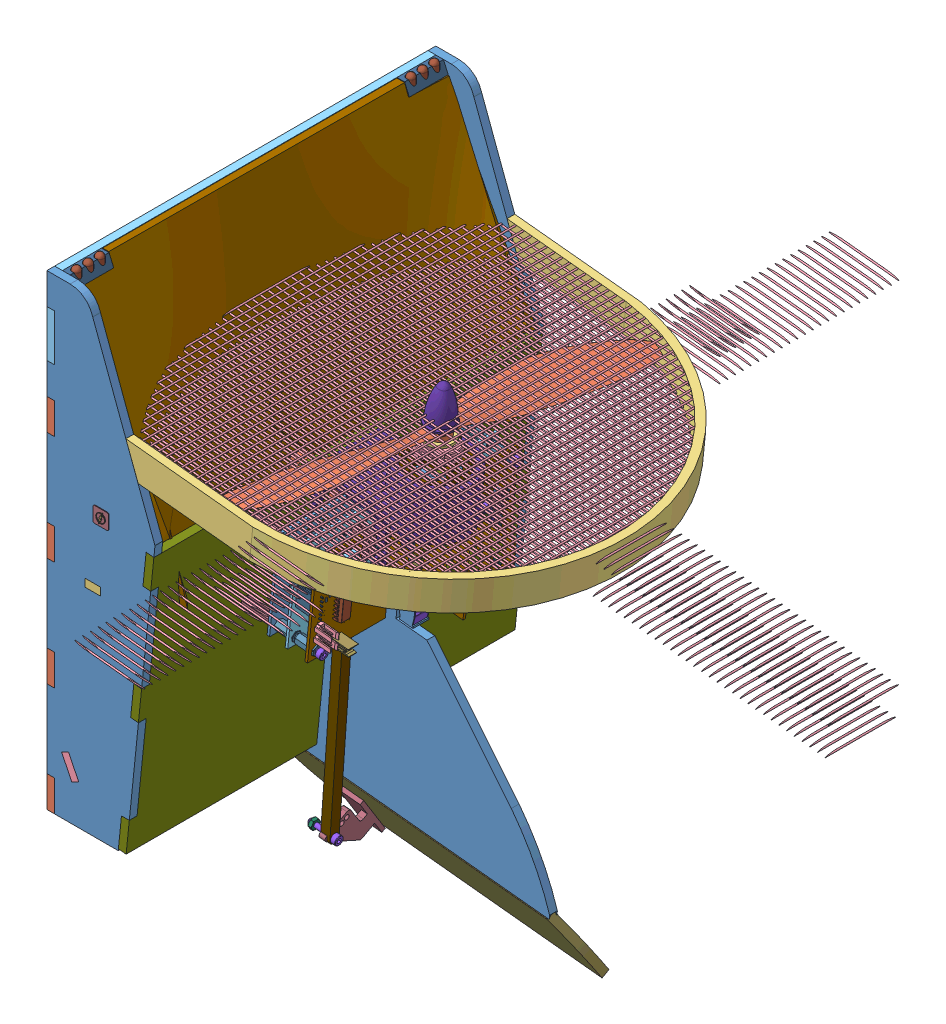
SolidWorks assembly AssTotaleSimu2, configuration Défaut. Lengths in mm. (continued)
Components (placement in the parent): (continued)
- AssStructSimu-1: AssStructSimu [Défaut] at (-125.7658 -1.8483 624.6548) x (1 0 0) z (0 0 -1) size (253.25 324.59 251.6) (continued)
  - AssCarte-1: AssCarte [Défaut] at (38.0121 147.1029 290.772) x (-0.101852 0.9948 0) z (0.9948 0.101852 0) size (66.52 130.57 98.72) (continued)
    - carte_onduleur_v3-1: carte_onduleur_v3 [Défaut] at (-131.8199 12.0892 20.7912) size (66.52 130.57 82.34) (continued)
      - U_DSPIC-1: U_DSPIC [Défaut] at (1.863 -2.61 0.803) size (7.92 35.56 7.75)
        - Open CASCADE STEP translator 6.8 1.17.1-1: Open CASCADE STEP translator 6.8 1.17.1 [Défaut] at origin size (7.92 35.56 7.75)
          - Body_1_4-1: Body_1_4 [Défaut] at (0 -0.2 4) x (1 0 0) z (0 -1 0) size (7.92 7.75 35.56)
      - C_DEC_DSPIC-1: C_DEC_DSPIC [Défaut] at (7.7 -8.8 -0.803) x (0 1 0) z (0 0 -1) size (2.34 1.04 0.5)
        - Open CASCADE STEP translator 6.8 1.6.1-1: Open CASCADE STEP translator 6.8 1.6.1 [Défaut] at origin size (2.34 1.04 0.5)
          - Body_1-1: Body_1 [Défaut] at origin size (2.29 1.04 0.43)
          - Pin_1-1: Pin_1 [Défaut] at (0.3048 0 0) x (-1 0 0) z (0 0 1) size (0.51 1.02 0.5)
          - Pin_2-1: Pin_2 [Défaut] at origin size (0.51 1.02 0.5)
      - IN-1: IN [Défaut] at (24.3 -5.3 0.803) x (0 1 0) z (0 0 1) size (10.21 15.56 26.9)
        - Open CASCADE STEP translator 6.8 1.19.1-1: Open CASCADE STEP translator 6.8 1.19.1 [Défaut] at origin size (10.21 15.56 26.9)
          - Body_1_3-1: Body_1_3 [Défaut] at (-13.5 1.8 3) x (0 1 0) z (1 0 0) size (15.56 26.9 10.21)
            - Imported-1: Imported [Défaut] at (2.0451 -4.5908 20.9802) size (8.6 15.9 10.16)
            - Imported-2: Imported [Défaut] at (-1.6683 9.1092 15.9802) x (0 0 1) z (-1 0 0) size (10.1 18.2 15.1)
              - Imported_2-1: Imported_2 [Défaut] at origin size (10.1 18.2 15.1)
              - Imported_3-1: Imported_3 [Défaut] at origin size (3.43 12.4 4.99)
              - Imported_4-1: Imported_4 [Défaut] at origin size (3.43 12.4 4.99)
              - Imported_5-1: Imported_5 [Défaut] at origin size (3.9 4.9 7)
              - Imported_6-1: Imported_6 [Défaut] at origin size (3.9 4.9 7)
              - Imported_7-1: Imported_7 [Défaut] at origin size (3.8 3.8 6.92)
              - Imported_8-1: Imported_8 [Défaut] at origin size (3.8 3.8 6.92)
              - Imported_9-1: Imported_9 [Défaut] at origin size (9 2.4 14.2)
      - CARTE_CMD-1: CARTE_CMD [Défaut] at (25 57.2 0.803) size (60.1 130 26.71)
        - Open CASCADE STEP translator 6.8 1.20.1-1: Open CASCADE STEP translator 6.8 1.20.1 [Défaut] at origin size (60.1 130 26.71)
          - Body_1_4-1: Body_1_4 [Défaut] at (-55 5 12) size (60.1 130 26.71)
            - 1_2-1: 1_2 [Défaut] at origin size (60.1 130 1.61)
            - 4-1: 4 [Défaut] at (23.6 -124.9 0.803) x (0 1 0) z (0 0 1) size (5 15.24 14.3)
              - =_[0_1_1_4]_2-1: =_[0_1_1_4]_2 [Défaut] at origin size (5 15.24 14.3)
                - 5-1: 5 [Défaut] at (0 -6.5 -13) x (0 1 0) z (0 0 -1) size (15.24 5 14.3)
            - 7-1: 7 [Défaut] at (23.6 -5 0.803) x (0 1 0) z (0 0 1) size (5 15.24 14.3)
              - =_[0_1_1_7]-1: =_[0_1_1_7] [Défaut] at origin size (5 15.24 14.3)
                - 5-1: 5 [Défaut] at (0 -6.5 -13) x (0 1 0) z (0 0 -1) size (15.24 5 14.3)
            - 10_2-1: 10_2 [Défaut] at (18.4 -115.6 0.803) size (25.4 7.92 7.75)
              - =_[0_1_1_9]-1: =_[0_1_1_9] [Défaut] at origin size (25.4 7.92 7.75)
                - 8-1: 8 [Défaut] at (11.2 4 0) x (0 1 0) z (1 0 0) size (7.92 7.75 25.4)
            - 13_2-1: 13_2 [Défaut] at (55.4 -114.7 0.803) x (-1 0 0) z (0 0 1) size (5 7.62 14.3)
              - =_[0_1_1_12]-1: =_[0_1_1_12] [Défaut] at origin size (5 7.62 14.3)
                - 11-1: 11 [Défaut] at (0 -2.5 11) x (0 -1 0) z (0 0 1) size (7.62 5 14.3)
            - 25-1: 25 [Défaut] at (56.9 -12.8 0.803) x (-1 0 0) z (0 0 1) size (16.02 47.26 11.05)
              - =_[0_1_1_15]_2-1: =_[0_1_1_15]_2 [Défaut] at origin size (16.02 47.26 11.05)
                - 23-1: 23 [Défaut] at (-36.5 21 4) x (0 -1 0) z (1 0 0) size (47.26 11.05 16.02)
                  - 14-1: 14 [Défaut] at (-7.4961 -1.5352 42.5833) size (42.58 6.55 16.01)
                  - 22-1: 22 [Défaut] at (19.3039 2.3748 37.905) x (-1 0 0) z (0 0 -1) size (10.36 6.14 15.24)
                    - 21-1: 21 [Défaut] at origin size (10.36 6.14 7.62)
                      - 19_2-1: 19_2 [Défaut] at origin size (10.36 6.14 2.54)
                        - 15-1: 15 [Défaut] at origin size (8.4 2.54 2.54)
                        - 16-1: 16 [Défaut] at (-0.0461 1.2682 1.27) x (0 0 -1) z (0.999998 -0.002105 0) size (1.95 5.07 7.58)
                      - 19_2-2: 19_2 [Défaut] at (0 0 -2.54) size (10.36 6.14 2.54)
                        - 15-1: 15 [Défaut] at origin size (8.4 2.54 2.54)
                        - 16-1: 16 [Défaut] at (-0.0461 1.2682 1.27) x (0 0 -1) z (0.999998 -0.002105 0) size (1.95 5.07 7.58)
                      - 19_2-3: 19_2 [Défaut] at (0 0 -5.08) size (10.36 6.14 2.54)
                        - 15-1: 15 [Défaut] at origin size (8.4 2.54 2.54)
                        - 16-1: 16 [Défaut] at (-0.0461 1.2682 1.27) x (0 0 -1) z (0.999998 -0.002105 0) size (1.95 5.07 7.58)
                    - 21-2: 21 [Défaut] at (0 0 -7.62) size (10.36 6.14 7.62)
                      - 19_2-1: 19_2 [Défaut] at origin size (10.36 6.14 2.54)
                        - 15-1: 15 [Défaut] at origin size (8.4 2.54 2.54)
                        - 16-1: 16 [Défaut] at (-0.0461 1.2682 1.27) x (0 0 -1) z (0.999998 -0.002105 0) size (1.95 5.07 7.58)
                      - 19_2-2: 19_2 [Défaut] at (0 0 -2.54) size (10.36 6.14 2.54)
                        - 15-1: 15 [Défaut] at origin size (8.4 2.54 2.54)
                        - 16-1: 16 [Défaut] at (-0.0461 1.2682 1.27) x (0 0 -1) z (0.999998 -0.002105 0) size (1.95 5.07 7.58)
                      - 19_2-3: 19_2 [Défaut] at (0 0 -5.08) size (10.36 6.14 2.54)
                        - 15-1: 15 [Défaut] at origin size (8.4 2.54 2.54)
                        - 16-1: 16 [Défaut] at (-0.0461 1.2682 1.27) x (0 0 -1) z (0.999998 -0.002105 0) size (1.95 5.07 7.58)
            - 31-1: 31 [Défaut] at (12.9 -104.5 0.803) size (6.76 3.64 4.37)
              - =_[0_1_1_24]-1: =_[0_1_1_24] [Défaut] at origin size (6.76 3.64 4.37)
                - 29-1: 29 [Défaut] at (-0.3 -2 0) size (6.76 3.64 4.37)
                  - =_[0_1_1_3]_3-1: =_[0_1_1_3]_3 [Défaut] at origin size (6 3.64 4.37)
                  - =_[0_1_1_4]_3-1: =_[0_1_1_4]_3 [Défaut] at origin size (0.38 1 0.67)
                  - =_[0_1_1_5]_3-1: =_[0_1_1_5]_3 [Défaut] at origin size (0.38 1 0.67)
            - 36-1: 36 [Défaut] at (28.6 -12.2 0.803) x (0 -1 0) z (0 0 1) size (2.34 1.04 0.5)
              - =_[0_1_1_30]-1: =_[0_1_1_30] [Défaut] at origin size (2.34 1.04 0.5)
                - 32_2-1: 32_2 [Défaut] at origin size (2.29 1.04 0.43)
                - 33_2-1: 33_2 [Défaut] at (0.3048 0 0) x (-1 0 0) z (0 0 1) size (0.51 1.02 0.5)
                - 34-1: 34 [Défaut] at origin size (0.51 1.02 0.5)
            - 38-1: 38 [Défaut] at (23.7 -12.2 0.803) x (0 -1 0) z (0 0 1) size (2.34 1.04 0.5)
              - =_[0_1_1_30]-1: =_[0_1_1_30] [Défaut] at origin size (2.34 1.04 0.5)
                - 32_2-1: 32_2 [Défaut] at origin size (2.29 1.04 0.43)
                - 33_2-1: 33_2 [Défaut] at (0.3048 0 0) x (-1 0 0) z (0 0 1) size (0.51 1.02 0.5)
                - 34-1: 34 [Défaut] at origin size (0.51 1.02 0.5)
            - 40_2-1: 40_2 [Défaut] at (26.2 -12.2 0.803) x (0 -1 0) z (0 0 1) size (2.34 1.04 0.5)
              - =_[0_1_1_30]-1: =_[0_1_1_30] [Défaut] at origin size (2.34 1.04 0.5)
                - 32_2-1: 32_2 [Défaut] at origin size (2.29 1.04 0.43)
                - 33_2-1: 33_2 [Défaut] at (0.3048 0 0) x (-1 0 0) z (0 0 1) size (0.51 1.02 0.5)
                - 34-1: 34 [Défaut] at origin size (0.51 1.02 0.5)
            - 42_2-1: 42_2 [Défaut] at (24.4 -119.2 0.803) size (2.34 1.04 0.5)
              - =_[0_1_1_30]-1: =_[0_1_1_30] [Défaut] at origin size (2.34 1.04 0.5)
                - 32_2-1: 32_2 [Défaut] at origin size (2.29 1.04 0.43)
                - 33_2-1: 33_2 [Défaut] at (0.3048 0 0) x (-1 0 0) z (0 0 1) size (0.51 1.02 0.5)
                - 34-1: 34 [Défaut] at origin size (0.51 1.02 0.5)
            - 45-1: 45 [Défaut] at (46.4 -125 0.803) size (5.08 5 14.3)
              - =_[0_1_1_38]-1: =_[0_1_1_38] [Défaut] at origin size (5.08 5 14.3)
                - 46-1: 46 [Défaut] at (1.2 0 11) size (5.08 5 14.3)
            - 48-1: 48 [Défaut] at (40.1 -125 0.803) size (5.08 5 14.3)
              - =_[0_1_1_41]-1: =_[0_1_1_41] [Défaut] at origin size (5.08 5 14.3)
                - 46-1: 46 [Défaut] at (1.2 0 11) size (5.08 5 14.3)
            - 51-1: 51 [Défaut] at (6.4 -119.9 0.803) x (0 1 0) z (0 0 1) size (15.24 2.54 7.37)
              - =_[0_1_1_43]-1: =_[0_1_1_43] [Défaut] at origin size (15.24 2.54 7.37)
                - 49_2-1: 49_2 [Défaut] at (6.5 0 0) x (1 0 0) z (0 -1 0) size (15.24 7.37 2.54)
            - 57_2-1: 57_2 [Défaut] at (50.8796 -121.1 -0.803) x (-1 0 0) z (0 0 -1) size (2.54 1.98 0.64)
              - =_[0_1_1_46]-1: =_[0_1_1_46] [Défaut] at origin size (2.54 1.98 0.64)
                - 52-1: 52 [Défaut] at origin size (2.54 1.14 0.58)
                - 53-1: 53 [Défaut] x (0 -1 0) z (0 0 1) size (0.43 0.51 0.38)
                - 54-1: 54 [Défaut] at (1.8796 1.8796 0) x (0 -1 0) z (0 0 1) size (0.43 0.51 0.38)
                - 55-1: 55 [Défaut] at (-0.9652 -2.8448 0) x (0 1 0) z (0 0 1) size (0.41 0.51 0.38)
            - 59_2-1: 59_2 [Défaut] at (43.6398 -120.995 -0.803) x (-1 0 0) z (0 0 -1) size (2.54 1.98 0.64)
              - =_[0_1_1_46]-1: =_[0_1_1_46] [Défaut] at origin size (2.54 1.98 0.64)
                - 52-1: 52 [Défaut] at origin size (2.54 1.14 0.58)
                - 53-1: 53 [Défaut] x (0 -1 0) z (0 0 1) size (0.43 0.51 0.38)
                - 54-1: 54 [Défaut] at (1.8796 1.8796 0) x (0 -1 0) z (0 0 1) size (0.43 0.51 0.38)
                - 55-1: 55 [Défaut] at (-0.9652 -2.8448 0) x (0 1 0) z (0 0 1) size (0.41 0.51 0.38)
            - 61_2-1: 61_2 [Défaut] at (47.6 -119.9 -0.803) x (-1 0 0) z (0 0 -1) size (2.34 1.04 0.5)
              - =_[0_1_1_30]-1: =_[0_1_1_30] [Défaut] at origin size (2.34 1.04 0.5)
                - 32_2-1: 32_2 [Défaut] at origin size (2.29 1.04 0.43)
                - 33_2-1: 33_2 [Défaut] at (0.3048 0 0) x (-1 0 0) z (0 0 1) size (0.51 1.02 0.5)
                - 34-1: 34 [Défaut] at origin size (0.51 1.02 0.5)
            - 63-1: 63 [Défaut] at (40.4 -119.9 -0.803) x (-1 0 0) z (0 0 -1) size (2.34 1.04 0.5)
              - =_[0_1_1_30]-1: =_[0_1_1_30] [Défaut] at origin size (2.34 1.04 0.5)
                - 32_2-1: 32_2 [Défaut] at origin size (2.29 1.04 0.43)
                - 33_2-1: 33_2 [Défaut] at (0.3048 0 0) x (-1 0 0) z (0 0 1) size (0.51 1.02 0.5)
                - 34-1: 34 [Défaut] at origin size (0.51 1.02 0.5)
            - 68-1: 68 [Défaut] at (47.7 -21.8 -0.803) x (0 1 0) z (0 0 -1) size (2.34 1.04 0.5)
              - =_[0_1_1_55]-1: =_[0_1_1_55] [Défaut] at origin size (2.34 1.04 0.5)
                - 64-1: 64 [Défaut] at origin size (2.29 1.04 0.43)
                - 65-1: 65 [Défaut] at (0.3048 0 0) x (-1 0 0) z (0 0 1) size (0.51 1.02 0.5)
                - 66-1: 66 [Défaut] at origin size (0.51 1.02 0.5)
            - 70-1: 70 [Défaut] at (47.6 -121.7 -0.803) x (-1 0 0) z (0 0 -1) size (2.34 1.04 0.5)
              - =_[0_1_1_30]-1: =_[0_1_1_30] [Défaut] at origin size (2.34 1.04 0.5)
                - 32_2-1: 32_2 [Défaut] at origin size (2.29 1.04 0.43)
                - 33_2-1: 33_2 [Défaut] at (0.3048 0 0) x (-1 0 0) z (0 0 1) size (0.51 1.02 0.5)
                - 34-1: 34 [Défaut] at origin size (0.51 1.02 0.5)
            - 72_2-1: 72_2 [Défaut] at (40.4 -121.5 -0.803) x (-1 0 0) z (0 0 -1) size (2.34 1.04 0.5)
              - =_[0_1_1_30]-1: =_[0_1_1_30] [Défaut] at origin size (2.34 1.04 0.5)
                - 32_2-1: 32_2 [Défaut] at origin size (2.29 1.04 0.43)
                - 33_2-1: 33_2 [Défaut] at (0.3048 0 0) x (-1 0 0) z (0 0 1) size (0.51 1.02 0.5)
                - 34-1: 34 [Défaut] at origin size (0.51 1.02 0.5)
            - 74_2-1: 74_2 [Défaut] at (47.7 -18.3 -0.803) x (0 1 0) z (0 0 -1) size (2.34 1.04 0.5)
              - =_[0_1_1_55]-1: =_[0_1_1_55] [Défaut] at origin size (2.34 1.04 0.5)
                - 64-1: 64 [Défaut] at origin size (2.29 1.04 0.43)
                - 65-1: 65 [Défaut] at (0.3048 0 0) x (-1 0 0) z (0 0 1) size (0.51 1.02 0.5)
                - 66-1: 66 [Défaut] at origin size (0.51 1.02 0.5)
            - 76_2-1: 76_2 [Défaut] at (45.5 -118.3 -0.803) x (1 0 0) z (0 0 -1) size (2.34 1.04 0.5)
              - =_[0_1_1_30]-1: =_[0_1_1_30] [Défaut] at origin size (2.34 1.04 0.5)
                - 32_2-1: 32_2 [Défaut] at origin size (2.29 1.04 0.43)
                - 33_2-1: 33_2 [Défaut] at (0.3048 0 0) x (-1 0 0) z (0 0 1) size (0.51 1.02 0.5)
                - 34-1: 34 [Défaut] at origin size (0.51 1.02 0.5)
            - 78_2-1: 78_2 [Défaut] at (38.2 -118.3 -0.803) x (1 0 0) z (0 0 -1) size (2.34 1.04 0.5)
              - =_[0_1_1_30]-1: =_[0_1_1_30] [Défaut] at origin size (2.34 1.04 0.5)
                - 32_2-1: 32_2 [Défaut] at origin size (2.29 1.04 0.43)
                - 33_2-1: 33_2 [Défaut] at (0.3048 0 0) x (-1 0 0) z (0 0 1) size (0.51 1.02 0.5)
                - 34-1: 34 [Défaut] at origin size (0.51 1.02 0.5)
            - 80_2-1: 80_2 [Défaut] at (28.6 -10.7 0.803) x (0 1 0) z (0 0 1) size (2.34 1.04 0.5)
              - =_[0_1_1_55]-1: =_[0_1_1_55] [Défaut] at origin size (2.34 1.04 0.5)
                - 64-1: 64 [Défaut] at origin size (2.29 1.04 0.43)
                - 65-1: 65 [Défaut] at (0.3048 0 0) x (-1 0 0) z (0 0 1) size (0.51 1.02 0.5)
                - 66-1: 66 [Défaut] at origin size (0.51 1.02 0.5)
            - 82_2-1: 82_2 [Défaut] at (23.7 -10.7 0.803) x (0 1 0) z (0 0 1) size (2.34 1.04 0.5)
              - =_[0_1_1_55]-1: =_[0_1_1_55] [Défaut] at origin size (2.34 1.04 0.5)
                - 64-1: 64 [Défaut] at origin size (2.29 1.04 0.43)
                - 65-1: 65 [Défaut] at (0.3048 0 0) x (-1 0 0) z (0 0 1) size (0.51 1.02 0.5)
                - 66-1: 66 [Défaut] at origin size (0.51 1.02 0.5)
            - 84-1: 84 [Défaut] at (26.2 -10.7 0.803) x (0 1 0) z (0 0 1) size (2.34 1.04 0.5)
              - =_[0_1_1_55]-1: =_[0_1_1_55] [Défaut] at origin size (2.34 1.04 0.5)
                - 64-1: 64 [Défaut] at origin size (2.29 1.04 0.43)
                - 65-1: 65 [Défaut] at (0.3048 0 0) x (-1 0 0) z (0 0 1) size (0.51 1.02 0.5)
                - 66-1: 66 [Défaut] at origin size (0.51 1.02 0.5)
            - 86-1: 86 [Défaut] at (23.0336 -119.2 0.803) x (-1 0 0) z (0 0 1) size (2.34 1.04 0.5)
              - =_[0_1_1_55]-1: =_[0_1_1_55] [Défaut] at origin size (2.34 1.04 0.5)
                - 64-1: 64 [Défaut] at origin size (2.29 1.04 0.43)
                - 65-1: 65 [Défaut] at (0.3048 0 0) x (-1 0 0) z (0 0 1) size (0.51 1.02 0.5)
                - 66-1: 66 [Défaut] at origin size (0.51 1.02 0.5)
            - 88-1: 88 [Défaut] at (14.1 -114.2 0.803) x (0 -1 0) z (0 0 1) size (2.34 1.04 0.5)
              - =_[0_1_1_55]-1: =_[0_1_1_55] [Défaut] at origin size (2.34 1.04 0.5)
                - 64-1: 64 [Défaut] at origin size (2.29 1.04 0.43)
                - 65-1: 65 [Défaut] at (0.3048 0 0) x (-1 0 0) z (0 0 1) size (0.51 1.02 0.5)
                - 66-1: 66 [Défaut] at origin size (0.51 1.02 0.5)
            - 90-1: 90 [Défaut] at (43.6 -107.8 -0.803) x (1 0 0) z (0 0 -1) size (2.34 1.04 0.5)
              - =_[0_1_1_55]-1: =_[0_1_1_55] [Défaut] at origin size (2.34 1.04 0.5)
                - 64-1: 64 [Défaut] at origin size (2.29 1.04 0.43)
                - 65-1: 65 [Défaut] at (0.3048 0 0) x (-1 0 0) z (0 0 1) size (0.51 1.02 0.5)
                - 66-1: 66 [Défaut] at origin size (0.51 1.02 0.5)
            - 92-1: 92 [Défaut] at (43.6 -106 -0.803) x (1 0 0) z (0 0 -1) size (2.34 1.04 0.5)
              - =_[0_1_1_55]-1: =_[0_1_1_55] [Défaut] at origin size (2.34 1.04 0.5)
                - 64-1: 64 [Défaut] at origin size (2.29 1.04 0.43)
                - 65-1: 65 [Défaut] at (0.3048 0 0) x (-1 0 0) z (0 0 1) size (0.51 1.02 0.5)
                - 66-1: 66 [Défaut] at origin size (0.51 1.02 0.5)
            - 175-1: 175 [Défaut] at (10 -21.7 0.803) x (0 -1 0) z (0 0 1) size (15 25.4 12.78)
              - =_[0_1_1_72]-1: =_[0_1_1_72] [Défaut] at origin size (15 25.4 12.78)
                - 173-1: 173 [Défaut] at (-1.4 -1 12) x (-1 0 0) z (0 1 0) size (15 12.78 25.4)
                  - board_1-1: board_1 [Défaut] at (-7.5 -1.57 12.5) size (15 1.57 25)
                  - hole_plating_20-1: hole_plating_20 [Défaut] at (-1.5 0 23.93) size (1.5 0.01 1.5)
                  - hole_plating_20-2: hole_plating_20 [Défaut] at (-1.5 0 21.39) size (1.5 0.01 1.5)
                  - hole_plating_20-3: hole_plating_20 [Défaut] at (-1.5 0 8.69) size (1.5 0.01 1.5)
                  - hole_plating_20-4: hole_plating_20 [Défaut] at (-1.5 -1.58 13.77) size (1.5 0.01 1.5)
                  - hole_plating_20-5: hole_plating_20 [Défaut] at (-1.5 0 16.31) size (1.5 0.01 1.5)
                  - hole_plating_20-6: hole_plating_20 [Défaut] at (-1.5 0 18.85) size (1.5 0.01 1.5)
                  - hole_plating_20-7: hole_plating_20 [Défaut] at (-1.5 0 13.77) size (1.5 0.01 1.5)
                  - hole_plating_20-8: hole_plating_20 [Défaut] at (-1.5 -1.58 11.23) size (1.5 0.01 1.5)
                  - hole_plating_20-9: hole_plating_20 [Défaut] at (-1.5 -1.58 18.85) size (1.5 0.01 1.5)
                  - hole_plating_20-10: hole_plating_20 [Défaut] at (-1.5 -1.58 6.15) size (1.5 0.01 1.5)
                  - hole_plating_20-11: hole_plating_20 [Défaut] at (-1.5 0 1.07) size (1.5 0.01 1.5)
                  - hole_plating_20-12: hole_plating_20 [Défaut] at (-1.5 -1.58 3.61) size (1.5 0.01 1.5)
                  - hole_plating_20-13: hole_plating_20 [Défaut] at (-1.5 -1.58 1.07) size (1.5 0.01 1.5)
                  - hole_plating_20-14: hole_plating_20 [Défaut] at (-1.5 -1.58 8.69) size (1.5 0.01 1.5)
                  - hole_plating_20-15: hole_plating_20 [Défaut] at (-1.5 -1.58 16.31) size (1.5 0.01 1.5)
                  - hole_plating_20-16: hole_plating_20 [Défaut] at (-1.5 0 11.23) size (1.5 0.01 1.5)
                  - hole_plating_20-17: hole_plating_20 [Défaut] at (-1.5 0 3.61) size (1.5 0.01 1.5)
                  - hole_plating_20-18: hole_plating_20 [Défaut] at (-1.5 -1.58 21.39) size (1.5 0.01 1.5)
                  - hole_plating_20-19: hole_plating_20 [Défaut] at (-1.5 0 6.15) size (1.5 0.01 1.5)
                  - hole_plating_20-20: hole_plating_20 [Défaut] at (-1.5 -1.58 23.93) size (1.5 0.01 1.5)
                  - Pin_Header_1x10_TH_Pitch_2.54mm_1-1: Pin_Header_1x10_TH_Pitch_2.54mm_1 [Défaut] at (-1.5 -1.5786 23.93) x (0 0 -1) z (0 -1 0) size (25.4 2.54 12.7)
                    - 124-1: 124 [Défaut] at origin size (25.4 2.54 2.8)
                      - =_[0_1_1_77]-1: =_[0_1_1_77] [Défaut] at origin size (2.54 2.54 2.8)
                      - =_[0_1_1_79]-1: =_[0_1_1_79] [Défaut] at origin size (2.54 2.54 2.8)
                      - =_[0_1_1_80]-1: =_[0_1_1_80] [Défaut] at origin size (2.54 2.54 2.8)
                      - =_[0_1_1_81]-1: =_[0_1_1_81] [Défaut] at origin size (2.54 2.54 2.8)
                      - =_[0_1_1_82]-1: =_[0_1_1_82] [Défaut] at origin size (2.54 2.54 2.8)
                      - =_[0_1_1_83]-1: =_[0_1_1_83] [Défaut] at origin size (2.54 2.54 2.8)
                      - =_[0_1_1_84]-1: =_[0_1_1_84] [Défaut] at origin size (2.54 2.54 2.8)
                      - =_[0_1_1_85]-1: =_[0_1_1_85] [Défaut] at origin size (2.54 2.54 2.8)
                      - =_[0_1_1_86]-1: =_[0_1_1_86] [Défaut] at origin size (2.54 2.54 2.8)
                      - =_[0_1_1_87]-1: =_[0_1_1_87] [Défaut] at origin size (2.54 2.54 2.8)
                    - 135-1: 135 [Défaut] at origin size (23.49 0.63 12.7)
                      - =_[0_1_1_88]-1: =_[0_1_1_88] [Défaut] at origin size (0.63 0.63 12.7)
                      - =_[0_1_1_90]-1: =_[0_1_1_90] [Défaut] at origin size (0.63 0.63 12.7)
                      - =_[0_1_1_91]-1: =_[0_1_1_91] [Défaut] at origin size (0.63 0.63 12.7)
                      - =_[0_1_1_92]-1: =_[0_1_1_92] [Défaut] at origin size (0.63 0.63 12.7)
                      - =_[0_1_1_93]-1: =_[0_1_1_93] [Défaut] at origin size (0.63 0.63 12.7)
                      - =_[0_1_1_94]-1: =_[0_1_1_94] [Défaut] at origin size (0.63 0.63 12.7)
                      - =_[0_1_1_95]-1: =_[0_1_1_95] [Défaut] at origin size (0.63 0.63 12.7)
                      - =_[0_1_1_96]-1: =_[0_1_1_96] [Défaut] at origin size (0.63 0.63 12.7)
                      - =_[0_1_1_97]-1: =_[0_1_1_97] [Défaut] at origin size (0.63 0.63 12.7)
                      - =_[0_1_1_98]-1: =_[0_1_1_98] [Défaut] at origin size (0.63 0.63 12.7)
                  - MPU-9250_1-1: MPU-9250_1 [Défaut] at (-8 0.05 12.5) x (-1 0 0) z (0 1 0) size (3 3 1.05)
                  - tantalum_10uF_1-1: tantalum_10uF_1 [Défaut] at (-13.167 0.1 10.9372) x (0 0 1) z (0 1 0) size (3.4 1.6 1.71)
                  - SOT23_5_1-1: SOT23_5_1 [Défaut] at (-7.475 -0.0136 21) x (0 0 1) z (0 1 0) size (3 3.2 0.92)
                  - RESC-0603_5-1: RESC-0603_5 [Défaut] at (-6.85 0 7.45) x (1 0 0) z (0 1 0) size (1.7 0.9 0.55)
                    - 143-1: 143 [Défaut] at origin size (1.7 0.9 0.55)
                      - =_[0_1_1_103]-1: =_[0_1_1_103] [Défaut] at origin size (0.4 0.9 0.53)
                      - =_[0_1_1_105]-1: =_[0_1_1_105] [Défaut] at origin size (0.4 0.9 0.53)
                      - =_[0_1_1_106]-1: =_[0_1_1_106] [Défaut] at origin size (1.64 0.9 0.52)
                    - 152-1: 152 [Défaut] at origin
                      - =_[0_1_1_107]-1: =_[0_1_1_107] [Défaut] at origin
                      - =_[0_1_1_109]-1: =_[0_1_1_109] [Défaut] at origin
                      - =_[0_1_1_110]-1: =_[0_1_1_110] [Défaut] at origin
                      - =_[0_1_1_111]-1: =_[0_1_1_111] [Défaut] at origin
                      - =_[0_1_1_112]-1: =_[0_1_1_112] [Défaut] at origin
                      - =_[0_1_1_113]-1: =_[0_1_1_113] [Défaut] at origin
                      - =_[0_1_1_114]-1: =_[0_1_1_114] [Défaut] at origin
                      - =_[0_1_1_115]-1: =_[0_1_1_115] [Défaut] at origin
                  - RESC-0603_5-2: RESC-0603_5 [Défaut] at (-9.85 0 16.05) x (1 0 0) z (0 1 0) size (1.7 0.9 0.55)
                    - 143-1: 143 [Défaut] at origin size (1.7 0.9 0.55)
                      - =_[0_1_1_103]-1: =_[0_1_1_103] [Défaut] at origin size (0.4 0.9 0.53)
                      - =_[0_1_1_105]-1: =_[0_1_1_105] [Défaut] at origin size (0.4 0.9 0.53)
                      - =_[0_1_1_106]-1: =_[0_1_1_106] [Défaut] at origin size (1.64 0.9 0.52)
                    - 152-1: 152 [Défaut] at origin
                      - =_[0_1_1_107]-1: =_[0_1_1_107] [Défaut] at origin
                      - =_[0_1_1_109]-1: =_[0_1_1_109] [Défaut] at origin
                      - =_[0_1_1_110]-1: =_[0_1_1_110] [Défaut] at origin
                      - =_[0_1_1_111]-1: =_[0_1_1_111] [Défaut] at origin
                      - =_[0_1_1_112]-1: =_[0_1_1_112] [Défaut] at origin
                      - =_[0_1_1_113]-1: =_[0_1_1_113] [Défaut] at origin
                      - =_[0_1_1_114]-1: =_[0_1_1_114] [Défaut] at origin
                      - =_[0_1_1_115]-1: =_[0_1_1_115] [Défaut] at origin
                  - RESC-0603_5-3: RESC-0603_5 [Défaut] at (-6.85 0 17.55) x (1 0 0) z (0 1 0) size (1.7 0.9 0.55)
                    - 143-1: 143 [Défaut] at origin size (1.7 0.9 0.55)
                      - =_[0_1_1_103]-1: =_[0_1_1_103] [Défaut] at origin size (0.4 0.9 0.53)
                      - =_[0_1_1_105]-1: =_[0_1_1_105] [Défaut] at origin size (0.4 0.9 0.53)
                      - =_[0_1_1_106]-1: =_[0_1_1_106] [Défaut] at origin size (1.64 0.9 0.52)
                    - 152-1: 152 [Défaut] at origin
                      - =_[0_1_1_107]-1: =_[0_1_1_107] [Défaut] at origin
                      - =_[0_1_1_109]-1: =_[0_1_1_109] [Défaut] at origin
                      - =_[0_1_1_110]-1: =_[0_1_1_110] [Défaut] at origin
                      - =_[0_1_1_111]-1: =_[0_1_1_111] [Défaut] at origin
                      - =_[0_1_1_112]-1: =_[0_1_1_112] [Défaut] at origin
                      - =_[0_1_1_113]-1: =_[0_1_1_113] [Défaut] at origin
                      - =_[0_1_1_114]-1: =_[0_1_1_114] [Défaut] at origin
                      - =_[0_1_1_115]-1: =_[0_1_1_115] [Défaut] at origin
                  - RESC-0603_5-4: RESC-0603_5 [Défaut] at (-6.85 0 16.05) x (1 0 0) z (0 1 0) size (1.7 0.9 0.55)
                    - 143-1: 143 [Défaut] at origin size (1.7 0.9 0.55)
                      - =_[0_1_1_103]-1: =_[0_1_1_103] [Défaut] at origin size (0.4 0.9 0.53)
                      - =_[0_1_1_105]-1: =_[0_1_1_105] [Défaut] at origin size (0.4 0.9 0.53)
                      - =_[0_1_1_106]-1: =_[0_1_1_106] [Défaut] at origin size (1.64 0.9 0.52)
                    - 152-1: 152 [Défaut] at origin
                      - =_[0_1_1_107]-1: =_[0_1_1_107] [Défaut] at origin
                      - =_[0_1_1_109]-1: =_[0_1_1_109] [Défaut] at origin
                      - =_[0_1_1_110]-1: =_[0_1_1_110] [Défaut] at origin
                      - =_[0_1_1_111]-1: =_[0_1_1_111] [Défaut] at origin
                      - =_[0_1_1_112]-1: =_[0_1_1_112] [Défaut] at origin
                      - =_[0_1_1_113]-1: =_[0_1_1_113] [Défaut] at origin
                      - =_[0_1_1_114]-1: =_[0_1_1_114] [Défaut] at origin
                      - =_[0_1_1_115]-1: =_[0_1_1_115] [Défaut] at origin
                  - RESC-0603_5-5: RESC-0603_5 [Défaut] at (-6.85 0 5.95) x (1 0 0) z (0 1 0) size (1.7 0.9 0.55)
                    - 143-1: 143 [Défaut] at origin size (1.7 0.9 0.55)
                      - =_[0_1_1_103]-1: =_[0_1_1_103] [Défaut] at origin size (0.4 0.9 0.53)
                      - =_[0_1_1_105]-1: =_[0_1_1_105] [Défaut] at origin size (0.4 0.9 0.53)
                      - =_[0_1_1_106]-1: =_[0_1_1_106] [Défaut] at origin size (1.64 0.9 0.52)
                    - 152-1: 152 [Défaut] at origin
                      - =_[0_1_1_107]-1: =_[0_1_1_107] [Défaut] at origin
                      - =_[0_1_1_109]-1: =_[0_1_1_109] [Défaut] at origin
                      - =_[0_1_1_110]-1: =_[0_1_1_110] [Défaut] at origin
                      - =_[0_1_1_111]-1: =_[0_1_1_111] [Défaut] at origin
                      - =_[0_1_1_112]-1: =_[0_1_1_112] [Défaut] at origin
                      - =_[0_1_1_113]-1: =_[0_1_1_113] [Défaut] at origin
                      - =_[0_1_1_114]-1: =_[0_1_1_114] [Défaut] at origin
                      - =_[0_1_1_115]-1: =_[0_1_1_115] [Défaut] at origin
                  - CAPC-0603-T0.9-BN_5-1: CAPC-0603-T0.9-BN_5 [Défaut] at (-9.85 0 8.95) x (1 0 0) z (0 1 0) size (1.7 0.9 0.9)
                    - =_[0_1_1_117]-1: =_[0_1_1_117] [Défaut] at origin size (1.7 0.9 0.9)
                    - 167-1: 167 [Défaut] at origin
                      - =_[0_1_1_118]-1: =_[0_1_1_118] [Défaut] at origin
                      - =_[0_1_1_120]-1: =_[0_1_1_120] [Défaut] at origin
                      - =_[0_1_1_121]-1: =_[0_1_1_121] [Défaut] at origin
                      - =_[0_1_1_122]-1: =_[0_1_1_122] [Défaut] at origin
                      - =_[0_1_1_123]-1: =_[0_1_1_123] [Défaut] at origin
                      - =_[0_1_1_124]-1: =_[0_1_1_124] [Défaut] at origin
                      - =_[0_1_1_125]-1: =_[0_1_1_125] [Défaut] at origin
                      - =_[0_1_1_126]-1: =_[0_1_1_126] [Défaut] at origin
                  - CAPC-0603-T0.9-BN_5-2: CAPC-0603-T0.9-BN_5 [Défaut] at (-6.85 0 8.95) x (1 0 0) z (0 1 0) size (1.7 0.9 0.9)
                    - =_[0_1_1_117]-1: =_[0_1_1_117] [Défaut] at origin size (1.7 0.9 0.9)
                    - 167-1: 167 [Défaut] at origin
                      - =_[0_1_1_118]-1: =_[0_1_1_118] [Défaut] at origin
                      - =_[0_1_1_120]-1: =_[0_1_1_120] [Défaut] at origin
                      - =_[0_1_1_121]-1: =_[0_1_1_121] [Défaut] at origin
                      - =_[0_1_1_122]-1: =_[0_1_1_122] [Défaut] at origin
                      - =_[0_1_1_123]-1: =_[0_1_1_123] [Défaut] at origin
                      - =_[0_1_1_124]-1: =_[0_1_1_124] [Défaut] at origin
                      - =_[0_1_1_125]-1: =_[0_1_1_125] [Défaut] at origin
                      - =_[0_1_1_126]-1: =_[0_1_1_126] [Défaut] at origin
                  - CAPC-0603-T0.9-BN_5-3: CAPC-0603-T0.9-BN_5 [Défaut] at (-6.85 0 19.05) x (1 0 0) z (0 1 0) size (1.7 0.9 0.9)
                    - =_[0_1_1_117]-1: =_[0_1_1_117] [Défaut] at origin size (1.7 0.9 0.9)
                    - 167-1: 167 [Défaut] at origin
                      - =_[0_1_1_118]-1: =_[0_1_1_118] [Défaut] at origin
                      - =_[0_1_1_120]-1: =_[0_1_1_120] [Défaut] at origin
                      - =_[0_1_1_121]-1: =_[0_1_1_121] [Défaut] at origin
                      - =_[0_1_1_122]-1: =_[0_1_1_122] [Défaut] at origin
                      - =_[0_1_1_123]-1: =_[0_1_1_123] [Défaut] at origin
                      - =_[0_1_1_124]-1: =_[0_1_1_124] [Défaut] at origin
                      - =_[0_1_1_125]-1: =_[0_1_1_125] [Défaut] at origin
                      - =_[0_1_1_126]-1: =_[0_1_1_126] [Défaut] at origin
                  - CAPC-0603-T0.9-BN_5-4: CAPC-0603-T0.9-BN_5 [Défaut] at (-9.85 0 7.45) x (1 0 0) z (0 1 0) size (1.7 0.9 0.9)
                    - =_[0_1_1_117]-1: =_[0_1_1_117] [Défaut] at origin size (1.7 0.9 0.9)
                    - 167-1: 167 [Défaut] at origin
                      - =_[0_1_1_118]-1: =_[0_1_1_118] [Défaut] at origin
                      - =_[0_1_1_120]-1: =_[0_1_1_120] [Défaut] at origin
                      - =_[0_1_1_121]-1: =_[0_1_1_121] [Défaut] at origin
                      - =_[0_1_1_122]-1: =_[0_1_1_122] [Défaut] at origin
                      - =_[0_1_1_123]-1: =_[0_1_1_123] [Défaut] at origin
                      - =_[0_1_1_124]-1: =_[0_1_1_124] [Défaut] at origin
                      - =_[0_1_1_125]-1: =_[0_1_1_125] [Défaut] at origin
                      - =_[0_1_1_126]-1: =_[0_1_1_126] [Défaut] at origin
                  - CAPC-0603-T0.9-BN_5-5: CAPC-0603-T0.9-BN_5 [Défaut] at (-9.85 0 17.55) x (1 0 0) z (0 1 0) size (1.7 0.9 0.9)
                    - =_[0_1_1_117]-1: =_[0_1_1_117] [Défaut] at origin size (1.7 0.9 0.9)
                    - 167-1: 167 [Défaut] at origin
                      - =_[0_1_1_118]-1: =_[0_1_1_118] [Défaut] at origin
                      - =_[0_1_1_120]-1: =_[0_1_1_120] [Défaut] at origin
                      - =_[0_1_1_121]-1: =_[0_1_1_121] [Défaut] at origin
                      - =_[0_1_1_122]-1: =_[0_1_1_122] [Défaut] at origin
                      - =_[0_1_1_123]-1: =_[0_1_1_123] [Défaut] at origin
                      - =_[0_1_1_124]-1: =_[0_1_1_124] [Défaut] at origin
                      - =_[0_1_1_125]-1: =_[0_1_1_125] [Défaut] at origin
                      - =_[0_1_1_126]-1: =_[0_1_1_126] [Défaut] at origin
            - 177-1: 177 [Défaut] at (52.1 -16.5 -0.803) x (1 0 0) z (0 0 -1) size (2.34 1.04 0.5)
              - =_[0_1_1_30]-1: =_[0_1_1_30] [Défaut] at origin size (2.34 1.04 0.5)
                - 32_2-1: 32_2 [Défaut] at origin size (2.29 1.04 0.43)
                - 33_2-1: 33_2 [Défaut] at (0.3048 0 0) x (-1 0 0) z (0 0 1) size (0.51 1.02 0.5)
                - 34-1: 34 [Défaut] at origin size (0.51 1.02 0.5)
            - 179-1: 179 [Défaut] at (22.5336 -121.5 -0.803) x (-1 0 0) z (0 0 -1) size (2.34 1.04 0.5)
              - =_[0_1_1_30]-1: =_[0_1_1_30] [Défaut] at origin size (2.34 1.04 0.5)
                - 32_2-1: 32_2 [Défaut] at origin size (2.29 1.04 0.43)
                - 33_2-1: 33_2 [Défaut] at (0.3048 0 0) x (-1 0 0) z (0 0 1) size (0.51 1.02 0.5)
                - 34-1: 34 [Défaut] at origin size (0.51 1.02 0.5)
            - 181-1: 181 [Défaut] at (48.6 -127 -0.803) x (-1 0 0) z (0 0 -1) size (2.34 1.04 0.5)
              - =_[0_1_1_30]-1: =_[0_1_1_30] [Défaut] at origin size (2.34 1.04 0.5)
                - 32_2-1: 32_2 [Défaut] at origin size (2.29 1.04 0.43)
                - 33_2-1: 33_2 [Défaut] at (0.3048 0 0) x (-1 0 0) z (0 0 1) size (0.51 1.02 0.5)
                - 34-1: 34 [Défaut] at origin size (0.51 1.02 0.5)
            - 183-1: 183 [Défaut] at (26.0189 -121.5 0.803) size (2.34 1.04 0.5)
              - =_[0_1_1_30]-1: =_[0_1_1_30] [Défaut] at origin size (2.34 1.04 0.5)
                - 32_2-1: 32_2 [Défaut] at origin size (2.29 1.04 0.43)
                - 33_2-1: 33_2 [Défaut] at (0.3048 0 0) x (-1 0 0) z (0 0 1) size (0.51 1.02 0.5)
                - 34-1: 34 [Défaut] at origin size (0.51 1.02 0.5)
            - 185-1: 185 [Défaut] at (30.3664 -19 -0.803) x (1 0 0) z (0 0 -1) size (2.34 1.04 0.5)
              - =_[0_1_1_30]-1: =_[0_1_1_30] [Défaut] at origin size (2.34 1.04 0.5)
                - 32_2-1: 32_2 [Défaut] at origin size (2.29 1.04 0.43)
                - 33_2-1: 33_2 [Défaut] at (0.3048 0 0) x (-1 0 0) z (0 0 1) size (0.51 1.02 0.5)
                - 34-1: 34 [Défaut] at origin size (0.51 1.02 0.5)
            - 187-1: 187 [Défaut] at (51.7 -114.3 -0.803) x (0 1 0) z (0 0 -1) size (2.34 1.04 0.5)
              - =_[0_1_1_30]-1: =_[0_1_1_30] [Défaut] at origin size (2.34 1.04 0.5)
                - 32_2-1: 32_2 [Défaut] at origin size (2.29 1.04 0.43)
                - 33_2-1: 33_2 [Défaut] at (0.3048 0 0) x (-1 0 0) z (0 0 1) size (0.51 1.02 0.5)
                - 34-1: 34 [Défaut] at origin size (0.51 1.02 0.5)
            - 189-1: 189 [Défaut] at (50 -114.3 -0.803) x (0 1 0) z (0 0 -1) size (2.34 1.04 0.5)
              - =_[0_1_1_30]-1: =_[0_1_1_30] [Défaut] at origin size (2.34 1.04 0.5)
                - 32_2-1: 32_2 [Défaut] at origin size (2.29 1.04 0.43)
                - 33_2-1: 33_2 [Défaut] at (0.3048 0 0) x (-1 0 0) z (0 0 1) size (0.51 1.02 0.5)
                - 34-1: 34 [Défaut] at origin size (0.51 1.02 0.5)
      - C2_1-1: C2_1 [Défaut] at (-20.6984 1.8 -0.803) x (1 0 0) z (0 0 -1) size (2.34 1.04 0.5)
        - Open CASCADE STEP translator 6.8 1.6.1-1: Open CASCADE STEP translator 6.8 1.6.1 [Défaut] at origin size (2.34 1.04 0.5)
          - Body_1-1: Body_1 [Défaut] at origin size (2.29 1.04 0.43)
          - Pin_1-1: Pin_1 [Défaut] at (0.3048 0 0) x (-1 0 0) z (0 0 1) size (0.51 1.02 0.5)
          - Pin_2-1: Pin_2 [Défaut] at origin size (0.51 1.02 0.5)
      - C2_2-1: C2_2 [Défaut] at (-24.2 1.8 -0.803) x (1 0 0) z (0 0 -1) size (2.34 1.04 0.5)
        - Open CASCADE STEP translator 6.8 1.6.1-1: Open CASCADE STEP translator 6.8 1.6.1 [Défaut] at origin size (2.34 1.04 0.5)
          - Body_1-1: Body_1 [Défaut] at origin size (2.29 1.04 0.43)
          - Pin_1-1: Pin_1 [Défaut] at (0.3048 0 0) x (-1 0 0) z (0 0 1) size (0.51 1.02 0.5)
          - Pin_2-1: Pin_2 [Défaut] at origin size (0.51 1.02 0.5)
      - C3_1-1: C3_1 [Défaut] at (-20.9176 -12.8 -0.803) x (1 0 0) z (0 0 -1) size (2.34 1.04 0.5)
        - Open CASCADE STEP translator 6.8 1.6.1-1: Open CASCADE STEP translator 6.8 1.6.1 [Défaut] at origin size (2.34 1.04 0.5)
          - Body_1-1: Body_1 [Défaut] at origin size (2.29 1.04 0.43)
          - Pin_1-1: Pin_1 [Défaut] at (0.3048 0 0) x (-1 0 0) z (0 0 1) size (0.51 1.02 0.5)
          - Pin_2-1: Pin_2 [Défaut] at origin size (0.51 1.02 0.5)
      - C3_2-1: C3_2 [Défaut] at (-24.4 -12.8 -0.803) x (1 0 0) z (0 0 -1) size (2.34 1.04 0.5)
        - Open CASCADE STEP translator 6.8 1.6.1-1: Open CASCADE STEP translator 6.8 1.6.1 [Défaut] at origin size (2.34 1.04 0.5)
          - Body_1-1: Body_1 [Défaut] at origin size (2.29 1.04 0.43)
          - Pin_1-1: Pin_1 [Défaut] at (0.3048 0 0) x (-1 0 0) z (0 0 1) size (0.51 1.02 0.5)
          - Pin_2-1: Pin_2 [Défaut] at origin size (0.51 1.02 0.5)
      - D_CUR-1: D_CUR [Défaut] at (-12.4432 3.85 -0.803) x (0 -1 0) z (0 0 -1) size (2.7 5.2 1.11)
        - Open CASCADE STEP translator 6.8 1.25.1-1: Open CASCADE STEP translator 6.8 1.25.1 [Défaut] at origin size (2.7 5.2 1.11)
          - Body_1_5-1: Body_1_5 [Défaut] at (1.2 -4 0) x (0 1 0) z (0 0 1) size (5.2 2.7 1.11)
            - =_[0_1_1_3]_4-1: =_[0_1_1_3]_4 [Défaut] at origin size (0.39 0.64 0.01)
            - =_[0_1_1_4]_4-1: =_[0_1_1_4]_4 [Défaut] at origin size (0.6 1.9 0.2)
            - =_[0_1_1_5]_4-1: =_[0_1_1_5]_4 [Défaut] at origin size (0.21 0.08 0.01)
            - =_[0_1_1_6]_2-1: =_[0_1_1_6]_2 [Défaut] at origin size (0.6 1.9 0.2)
            - =_[0_1_1_7]_2-1: =_[0_1_1_7]_2 [Défaut] at origin size (0.46 0.68 0.01)
            - =_[0_1_1_8]_2-1: =_[0_1_1_8]_2 [Défaut] at origin size (0.38 0.66 0.01)
            - =_[0_1_1_9]-1: =_[0_1_1_9] [Défaut] at origin size (0.2 0.62 0.01)
            - =_[0_1_1_10]-1: =_[0_1_1_10] [Défaut] at origin size (4 2.7 1.1)
            - =_[0_1_1_11]-1: =_[0_1_1_11] [Défaut] at origin size (0.46 0.63 0.01)
            - =_[0_1_1_12]-1: =_[0_1_1_12] [Défaut] at origin size (0.56 0.68 0.01)
      - RC1_1-1: RC1_1 [Défaut] at (-20.7176 8.1 -0.803) x (1 0 0) z (0 0 -1) size (2.34 1.04 0.5)
        - Open CASCADE STEP translator 6.8 1.12.1-1: Open CASCADE STEP translator 6.8 1.12.1 [Défaut] at origin size (2.34 1.04 0.5)
          - Body_1_3-1: Body_1_3 [Défaut] at origin size (2.29 1.04 0.43)
          - Pin_1_2-1: Pin_1_2 [Défaut] at (0.3048 0 0) x (-1 0 0) z (0 0 1) size (0.51 1.02 0.5)
          - Pin_2_2-1: Pin_2_2 [Défaut] at origin size (0.51 1.02 0.5)
      - RC1_2-1: RC1_2 [Défaut] at (-22 8.1 -0.803) x (-1 0 0) z (0 0 -1) size (2.34 1.04 0.5)
        - Open CASCADE STEP translator 6.8 1.12.1-1: Open CASCADE STEP translator 6.8 1.12.1 [Défaut] at origin size (2.34 1.04 0.5)
          - Body_1_3-1: Body_1_3 [Défaut] at origin size (2.29 1.04 0.43)
          - Pin_1_2-1: Pin_1_2 [Défaut] at (0.3048 0 0) x (-1 0 0) z (0 0 1) size (0.51 1.02 0.5)
          - Pin_2_2-1: Pin_2_2 [Défaut] at origin size (0.51 1.02 0.5)
      - RC2_1-1: RC2_1 [Défaut] at (-20.716 0.243 -0.803) x (1 0 0) z (0 0 -1) size (2.34 1.04 0.5)
        - Open CASCADE STEP translator 6.8 1.12.1-1: Open CASCADE STEP translator 6.8 1.12.1 [Défaut] at origin size (2.34 1.04 0.5)
          - Body_1_3-1: Body_1_3 [Défaut] at origin size (2.29 1.04 0.43)
          - Pin_1_2-1: Pin_1_2 [Défaut] at (0.3048 0 0) x (-1 0 0) z (0 0 1) size (0.51 1.02 0.5)
          - Pin_2_2-1: Pin_2_2 [Défaut] at origin size (0.51 1.02 0.5)
      - RC2_2-1: RC2_2 [Défaut] at (-22 0.18 -0.803) x (-1 0 0) z (0 0 -1) size (2.34 1.04 0.5)
        - Open CASCADE STEP translator 6.8 1.12.1-1: Open CASCADE STEP translator 6.8 1.12.1 [Défaut] at origin size (2.34 1.04 0.5)
          - Body_1_3-1: Body_1_3 [Défaut] at origin size (2.29 1.04 0.43)
          - Pin_1_2-1: Pin_1_2 [Défaut] at (0.3048 0 0) x (-1 0 0) z (0 0 1) size (0.51 1.02 0.5)
